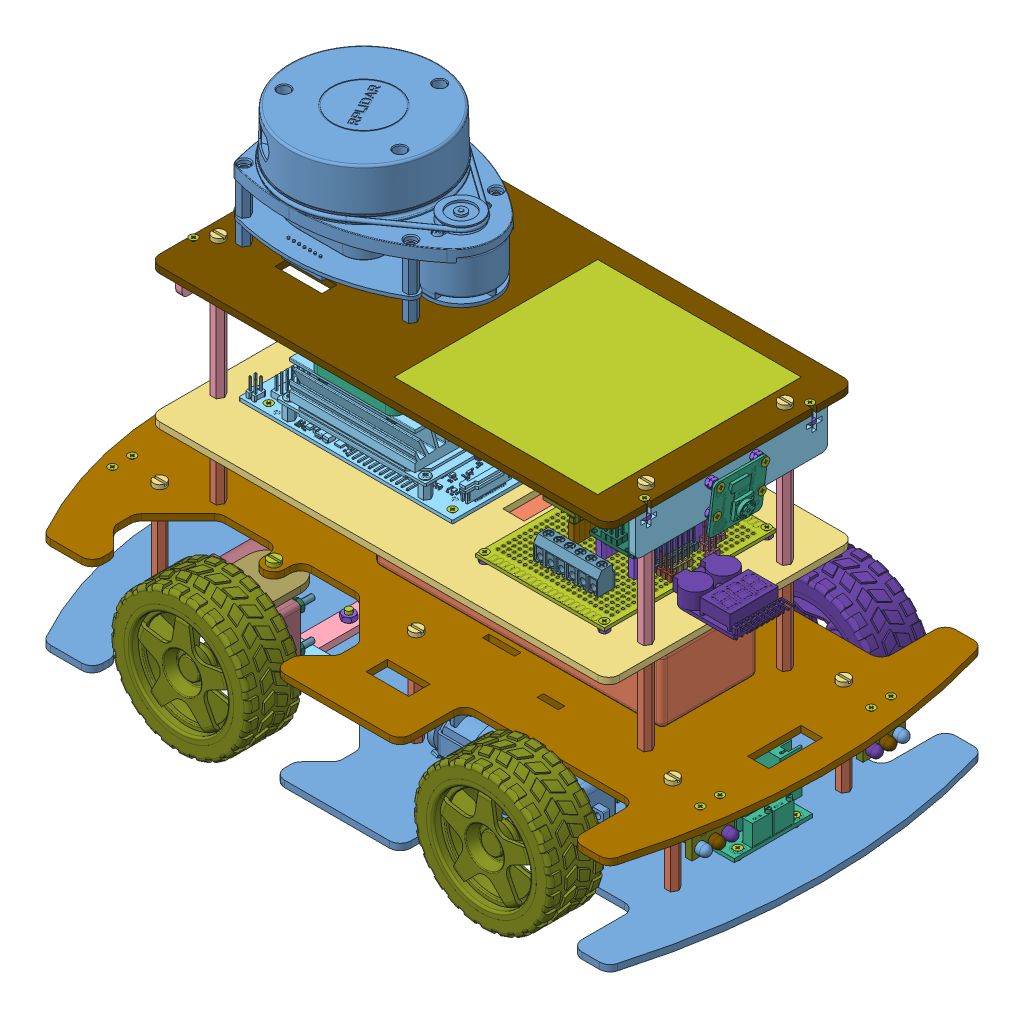
SolidWorks assembly Nigel - Motion Analysis, configuration Default. Lengths in mm. (continued)
Mates (geometry in assembly coordinates): (continued)
- Coincident280: coincident: circle of Platform 2-1; cone of M2x10 Bolt-16 through (137.5 46.8 -44.6) axis (0 -1 0)
- Concentric255: concentric: cylinder of M2x10 Bolt-16 through (137.5 47.6723 -44.6) axis (0 1 0) radius 1; cylinder of M2 Nut-16 through (137.5 40.5 -44.6) axis (0 -1 0) radius 1
- Coincident281: coincident: plane of LED Mount-4 through (139 40.5 -40) normal (0 -1 0); plane of M2 Nut-16 through (137.5 40.5 -44.6) normal (0 1 0)
- Concentric256: concentric: cylinder of Platform 3-1 through (-80 89 29) axis (0 -1 0) radius 1.1; cylinder of M2x10 Bolt-17 through (-80 94.4673 29) axis (0 1 0) radius 1
- Coincident282: coincident: circle of Jetson Nano B01-1; cone of M2x10 Bolt-17 through (-80 93.595 29) axis (0 -1 0)
- Concentric257: concentric: cylinder of Platform 3-1 through (-80 89 -29) axis (0 -1 0) radius 1.1; cylinder of M2x10 Bolt-18 through (-80 94.4673 -29) axis (0 1 0) radius 1
- Coincident283: coincident: circle of Jetson Nano B01-1; cone of M2x10 Bolt-18 through (-80 93.595 -29) axis (0 -1 0)
- Concentric258: concentric: cylinder of Platform 3-1 through (6 89 29) axis (0 -1 0) radius 1.1; cylinder of M2x10 Bolt-19 through (6 94.4673 29) axis (0 1 0) radius 1
- Coincident284: coincident: circle of Jetson Nano B01-1; cone of M2x10 Bolt-19 through (6 93.595 29) axis (0 -1 0)
- Concentric259: concentric: cylinder of Platform 3-1 through (6 89 -29) axis (0 -1 0) radius 1.1; cylinder of M2x10 Bolt-20 through (6 94.4673 -29) axis (0 1 0) radius 1
- Coincident285: coincident: circle of Jetson Nano B01-1; cone of M2x10 Bolt-20 through (6 93.595 -29) axis (0 -1 0)
- Concentric260: concentric: cylinder of M2x10 Bolt-17 through (-80 94.4673 29) axis (0 1 0) radius 1; cylinder of M2 Nut-17 through (-80 86 29) axis (0 -1 0) radius 1
- Coincident286: coincident: plane of Platform 3-1 through (0 86 0) normal (0 -1 0); plane of M2 Nut-17 through (-80 86 29) normal (0 1 0)
- Concentric261: concentric: cylinder of M2x10 Bolt-18 through (-80 94.4673 -29) axis (0 1 0) radius 1; cylinder of M2 Nut-18 through (-80 86 -29) axis (0 -1 0) radius 1
- Coincident287: coincident: plane of Platform 3-1 through (0 86 0) normal (0 -1 0); plane of M2 Nut-18 through (-80 86 -29) normal (0 1 0)
- Concentric262: concentric: cylinder of M2x10 Bolt-19 through (6 94.4673 29) axis (0 1 0) radius 1; cylinder of M2 Nut-19 through (6 86 29) axis (0 -1 0) radius 1
- Coincident288: coincident: plane of Platform 3-1 through (0 86 0) normal (0 -1 0); plane of M2 Nut-19 through (6 86 29) normal (0 1 0)
- Concentric263: concentric: cylinder of M2x10 Bolt-20 through (6 94.4673 -29) axis (0 1 0) radius 1; cylinder of M2 Nut-20 through (6 86 -29) axis (0 -1 0) radius 1
- Coincident289: coincident: plane of Platform 3-1 through (0 86 0) normal (0 -1 0); plane of M2 Nut-20 through (6 86 -29) normal (0 1 0)
- Concentric264: concentric: cylinder of Platform 4-1 through (-100 152 32.5) axis (0 -1 0) radius 1.6; cylinder of M3x8 Bolt-17 through (-100 144 32.5) axis (0 1 0) radius 1.5
- Coincident290: coincident: plane of Platform 4-1 through (0 152 0) normal (0 1 0); plane of M3x8 Bolt-17 through (-100 152 32.5) normal (0 -1 0)
- Concentric265: concentric: cylinder of Platform 4-1 through (-100 152 -32.5) axis (0 -1 0) radius 1.6; cylinder of M3x8 Bolt-18 through (-100 144 -32.5) axis (0 1 0) radius 1.5
- Coincident291: coincident: plane of Platform 4-1 through (0 152 0) normal (0 1 0); plane of M3x8 Bolt-18 through (-100 152 -32.5) normal (0 -1 0)
- Concentric266: concentric: cylinder of Platform 4-1 through (100 152 32.5) axis (0 -1 0) radius 1.6; cylinder of M3x8 Bolt-19 through (100 144 32.5) axis (0 1 0) radius 1.5
- Coincident292: coincident: plane of Platform 4-1 through (0 152 0) normal (0 1 0); plane of M3x8 Bolt-19 through (100 152 32.5) normal (0 -1 0)
- Concentric267: concentric: cylinder of Platform 4-1 through (100 152 -32.5) axis (0 -1 0) radius 1.6; cylinder of M3x8 Bolt-20 through (100 144 -32.5) axis (0 1 0) radius 1.5
- Coincident293: coincident: plane of Platform 4-1 through (0 152 0) normal (0 1 0); plane of M3x8 Bolt-20 through (100 152 -32.5) normal (0 -1 0)
- Concentric268: concentric: cylinder of Platform 4-1 through (-92.5 152 28) axis (0 -1 0) radius 1.35; cylinder of M2.5x8 Bolt-1 through (-92.5 147.1277 28) axis (0 -1 0) radius 1.25
- Coincident294: coincident: circle of Platform 4-1; cone of M2.5x8 Bolt-1 through (-92.5 148 28) axis (0 1 0)
- Concentric269: concentric: cylinder of Platform 4-1 through (-92.5 152 -28) axis (0 -1 0) radius 1.35; cylinder of M2.5x8 Bolt-2 through (-92.5 147.1277 -28) axis (0 -1 0) radius 1.25
- Coincident295: coincident: circle of Platform 4-1; cone of M2.5x8 Bolt-2 through (-92.5 148 -28) axis (0 1 0)
- Concentric270: concentric: cylinder of Platform 4-1 through (-22.5 152 20) axis (0 -1 0) radius 1.35; cylinder of M2.5x8 Bolt-3 through (-22.5 147.1277 20) axis (0 -1 0) radius 1.25
- Coincident296: coincident: circle of Platform 4-1; cone of M2.5x8 Bolt-3 through (-22.5 148 20) axis (0 1 0)
- Concentric271: concentric: cylinder of Platform 4-1 through (-22.5 152 -20) axis (0 -1 0) radius 1.35; cylinder of M2.5x8 Bolt-4 through (-22.5 147.1277 -20) axis (0 -1 0) radius 1.25
- Coincident297: coincident: circle of Platform 4-1; cone of M2.5x8 Bolt-4 through (-22.5 148 -20) axis (0 1 0)
- Concentric272: concentric: cylinder of RPLIDAR Adapter-1 through (-57.5 150.2284 -46.5) axis (0 -1 0) radius 1; cylinder of M2x10 Bolt-21 through (-57.5 144.1277 -46.5) axis (0 -1 0) radius 1
- Coincident298: coincident: circle of RPLIDAR Adapter-1; cone of M2x10 Bolt-21 through (-57.5 145 -46.5) axis (0 1 0)
- Concentric273: concentric: cylinder of RPLIDAR Adapter-1 through (-71.5 150.2284 -46.5) axis (0 -1 0) radius 1; cylinder of M2x10 Bolt-22 through (-71.5 144.1277 -46.5) axis (0 -1 0) radius 1
- Coincident299: coincident: circle of RPLIDAR Adapter-1; cone of M2x10 Bolt-22 through (-71.5 145 -46.5) axis (0 1 0)
- Concentric274: concentric: cylinder of RPLIDAR Adapter-1 through (-57.5 150.2284 -28) axis (0 -1 0) radius 1; cylinder of M2x10 Bolt-23 through (-57.5 144.1277 -28) axis (0 -1 0) radius 1
- Coincident300: coincident: circle of RPLIDAR Adapter-1; cone of M2x10 Bolt-23 through (-57.5 145 -28) axis (0 1 0)
- Concentric275: concentric: cylinder of RPLIDAR Adapter-1 through (-71.5 150.2284 -28) axis (0 -1 0) radius 1; cylinder of M2x10 Bolt-24 through (-71.5 144.1277 -28) axis (0 -1 0) radius 1
- Coincident301: coincident: circle of RPLIDAR Adapter-1; cone of M2x10 Bolt-24 through (-71.5 145 -28) axis (0 1 0)
- Concentric276: concentric: cylinder of M2x10 Bolt-21 through (-57.5 144.1277 -46.5) axis (0 -1 0) radius 1; cylinder of M2 Nut-21 through (-57.5 153.6 -46.5) axis (0 -1 0) radius 1
- Coincident302: coincident: plane of Platform 4-1 through (0 152 0) normal (0 1 0); plane of M2 Nut-21 through (-57.5 152 -46.5) normal (0 -1 0)
- Concentric277: concentric: cylinder of M2x10 Bolt-22 through (-71.5 144.1277 -46.5) axis (0 -1 0) radius 1; cylinder of M2 Nut-22 through (-71.5 153.6 -46.5) axis (0 -1 0) radius 1
- Coincident303: coincident: plane of Platform 4-1 through (0 152 0) normal (0 1 0); plane of M2 Nut-22 through (-71.5 152 -46.5) normal (0 -1 0)
- Concentric278: concentric: cylinder of M2x10 Bolt-23 through (-57.5 144.1277 -28) axis (0 -1 0) radius 1; cylinder of M2 Nut-23 through (-57.5 153.6 -28) axis (0 -1 0) radius 1
- Coincident304: coincident: plane of Platform 4-1 through (0 152 0) normal (0 1 0); plane of M2 Nut-23 through (-57.5 152 -28) normal (0 -1 0)
- Concentric279: concentric: cylinder of M2x10 Bolt-24 through (-71.5 144.1277 -28) axis (0 -1 0) radius 1; cylinder of M2 Nut-24 through (-71.5 153.6 -28) axis (0 -1 0) radius 1
- Coincident305: coincident: plane of Platform 4-1 through (0 152 0) normal (0 1 0); plane of M2 Nut-24 through (-71.5 152 -28) normal (0 -1 0)
- Tangent1: tangent: plane of Platform 4-1 through (-104.5 152 -39.8) normal (-1 0 0); cylinder of M2x10 Bolt-25 through (-105.5 153.6723 -38.7) axis (0 1 0) radius 1
- Distance33: distance = 0.1 mm: cylinder of M2x10 Bolt-25 through (-105.5 153.6723 -38.7) axis (0 1 0) radius 1; plane of Platform 4-1 through (-107.5 152 -39.8) normal (0 0 1)
- Distance34: distance = 3.7 mm: plane of M2x10 Bolt-25 through (-105.5 142.8 -38.7) normal (0 -1 0); plane of Front Camera Mount-1 through (-104.5 146.5 -37.6) normal (0 -1 0)
- Parallel23: parallel: plane of Front Camera Mount-1 through (-107.5 140.25 0) normal (-1 0 0); plane of M2x10 Bolt-25 through (-105.5 152.8 -38.7) normal (1 0 0)
- Tangent3: tangent: plane of Platform 4-1 through (-104.5 152 39.8) normal (-1 0 0); cylinder of M2x10 Bolt-26 through (-105.5 153.6723 38.7) axis (0 1 0) radius 1
- Distance35: distance = 0.1 mm: cylinder of M2x10 Bolt-26 through (-105.5 153.6723 38.7) axis (0 1 0) radius 1; plane of Platform 4-1 through (-104.5 152 37.6) normal (0 0 1)
- Distance36: distance = 3.7 mm: plane of M2x10 Bolt-26 through (-105.5 142.8 38.7) normal (0 -1 0); plane of Front Camera Mount-1 through (-104.5 146.5 42.3) normal (0 -1 0)
- Parallel24: parallel: plane of Front Camera Mount-1 through (-107.5 140.25 0) normal (-1 0 0); plane of M2x10 Bolt-26 through (-105.5 152.8 38.7) normal (1 0 0)
- Concentric280: concentric: cylinder of M2x10 Bolt-25 through (-105.5 153.6723 -38.7) axis (0 1 0) radius 1; cylinder of M2 Nut-25 through (-105.5 146.5 -38.7) axis (0 -1 0) radius 1
- Coincident310: coincident: plane of Front Camera Mount-1 through (-104.5 146.5 -37.6) normal (0 -1 0); plane of M2 Nut-25 through (-105.5 146.5 -38.7) normal (0 1 0)
- Concentric281: concentric: cylinder of M2x10 Bolt-26 through (-105.5 153.6723 38.7) axis (0 1 0) radius 1; cylinder of M2 Nut-26 through (-105.5 146.5 38.7) axis (0 -1 0) radius 1
- Coincident311: coincident: plane of Front Camera Mount-1 through (-104.5 146.5 42.3) normal (0 -1 0); plane of M2 Nut-26 through (-105.5 146.5 38.7) normal (0 1 0)
- Tangent5: tangent: plane of Platform 4-1 through (104.5 152 39.8) normal (1 0 0); cylinder of M2x10 Bolt-27 through (105.5 153.6723 38.7) axis (0 1 0) radius 1
- Distance37: distance = 0.1 mm: cylinder of M2x10 Bolt-27 through (105.5 153.6723 38.7) axis (0 1 0) radius 1; plane of Platform 4-1 through (107.5 152 39.8) normal (0 0 -1)
- Distance38: distance = 3.7 mm: plane of M2x10 Bolt-27 through (105.5 142.8 38.7) normal (0 -1 0); plane of Rear Camera Mount-1 through (107.5 146.5 37.6) normal (0 -1 0)
- Parallel25: parallel: plane of Rear Camera Mount-1 through (107.5 140.25 0) normal (1 0 0); plane of M2x10 Bolt-27 through (105.5 152.8 38.7) normal (1 0 0)
- Tangent7: tangent: plane of Platform 4-1 through (104.5 152 -39.8) normal (1 0 0); cylinder of M2x10 Bolt-28 through (105.5 153.6723 -38.7) axis (0 1 0) radius 1
- Distance39: distance = 0.1 mm: cylinder of M2x10 Bolt-28 through (105.5 153.6723 -38.7) axis (0 1 0) radius 1; plane of Platform 4-1 through (104.5 152 -37.6) normal (0 0 -1)
- Distance40: distance = 3.7 mm: plane of M2x10 Bolt-28 through (105.5 142.8 -38.7) normal (0 -1 0); plane of Rear Camera Mount-1 through (107.5 146.5 -42.3) normal (0 -1 0)
- Parallel26: parallel: plane of Rear Camera Mount-1 through (107.5 140.25 0) normal (1 0 0); plane of M2x10 Bolt-28 through (105.5 152.8 -38.7) normal (1 0 0)
- Concentric282: concentric: cylinder of M2x10 Bolt-27 through (105.5 153.6723 38.7) axis (0 1 0) radius 1; cylinder of M2 Nut-27 through (105.5 146.5 38.7) axis (0 -1 0) radius 1
- Coincident316: coincident: plane of Rear Camera Mount-1 through (107.5 146.5 37.6) normal (0 -1 0); plane of M2 Nut-27 through (105.5 146.5 38.7) normal (0 1 0)
- Concentric283: concentric: cylinder of M2x10 Bolt-28 through (105.5 153.6723 -38.7) axis (0 1 0) radius 1; cylinder of M2 Nut-28 through (105.5 146.5 -38.7) axis (0 -1 0) radius 1
- Coincident317: coincident: plane of Rear Camera Mount-1 through (107.5 146.5 -42.3) normal (0 -1 0); plane of M2 Nut-28 through (105.5 146.5 -38.7) normal (0 1 0)
- Concentric284: concentric: cylinder of Front Camera Mount-1 through (-104.5 146.5 -10.5) axis (-1 0 0) radius 1.1; cylinder of M2x10 Bolt-29 through (-113.8723 146.5 -10.5) axis (-1 0 0) radius 1
- Concentric285: concentric: cylinder of Front Camera Mount-1 through (-104.5 146.5 10.5) axis (-1 0 0) radius 1.1; cylinder of M2x10 Bolt-30 through (-113.8723 146.5 10.5) axis (-1 0 0) radius 1
- Concentric286: concentric: cylinder of Front Camera Mount-1 through (-104.5 134 -10.5) axis (-1 0 0) radius 1.1; cylinder of M2x10 Bolt-31 through (-112.2723 134 -10.5) axis (-1 0 0) radius 1
- Concentric287: concentric: cylinder of Front Camera Mount-1 through (-104.5 134 10.5) axis (-1 0 0) radius 1.1; cylinder of M2x10 Bolt-32 through (-112.2723 134 10.5) axis (-1 0 0) radius 1
- Concentric288: concentric: cylinder of M2x10 Bolt-29 through (-113.8723 146.5 -10.5) axis (-1 0 0) radius 1; cylinder of M2 Nut-29 through (-102.9 146.5 -10.5) axis (-1 0 0) radius 1
- Coincident322: coincident: plane of Front Camera Mount-1 through (-104.5 140.25 0) normal (1 0 0); plane of M2 Nut-29 through (-104.5 146.5 -10.5) normal (-1 0 0)
- Concentric289: concentric: cylinder of M2x10 Bolt-30 through (-113.8723 146.5 10.5) axis (-1 0 0) radius 1; cylinder of M2 Nut-30 through (-102.9 146.5 10.5) axis (-1 0 0) radius 1
- Coincident323: coincident: plane of Front Camera Mount-1 through (-104.5 140.25 0) normal (1 0 0); plane of M2 Nut-30 through (-104.5 146.5 10.5) normal (-1 0 0)
- Concentric290: concentric: cylinder of M2x10 Bolt-31 through (-112.2723 134 -10.5) axis (-1 0 0) radius 1; cylinder of M2 Nut-31 through (-102.9 134 -10.5) axis (-1 0 0) radius 1
- Coincident324: coincident: plane of Front Camera Mount-1 through (-104.5 140.25 0) normal (1 0 0); plane of M2 Nut-31 through (-104.5 134 -10.5) normal (-1 0 0)
- Concentric291: concentric: cylinder of M2x10 Bolt-32 through (-112.2723 134 10.5) axis (-1 0 0) radius 1; cylinder of M2 Nut-32 through (-102.9 134 10.5) axis (-1 0 0) radius 1
- Coincident325: coincident: plane of Front Camera Mount-1 through (-104.5 140.25 0) normal (1 0 0); plane of M2 Nut-32 through (-104.5 134 10.5) normal (-1 0 0)
- Concentric292: concentric: cylinder of Rear Camera Mount-1 through (107.5 146.5 10.5) axis (-1 0 0) radius 1.1; cylinder of M2x10 Bolt-33 through (113.8723 146.5 10.5) axis (1 0 0) radius 1
- Concentric293: concentric: cylinder of Rear Camera Mount-1 through (107.5 146.5 -10.5) axis (-1 0 0) radius 1.1; cylinder of M2x10 Bolt-34 through (113.8723 146.5 -10.5) axis (1 0 0) radius 1
- Concentric294: concentric: cylinder of Rear Camera Mount-1 through (107.5 134 10.5) axis (-1 0 0) radius 1.1; cylinder of M2x10 Bolt-35 through (112.2723 134 10.5) axis (1 0 0) radius 1
- Concentric295: concentric: cylinder of Rear Camera Mount-1 through (107.5 134 -10.5) axis (-1 0 0) radius 1.1; cylinder of M2x10 Bolt-36 through (112.2723 134 -10.5) axis (1 0 0) radius 1
- Concentric296: concentric: cylinder of M2x10 Bolt-33 through (113.8723 146.5 10.5) axis (1 0 0) radius 1; cylinder of M2 Nut-33 through (104.5 146.5 10.5) axis (-1 0 0) radius 1
- Coincident330: coincident: plane of Rear Camera Mount-1 through (104.5 140.25 0) normal (-1 0 0); plane of M2 Nut-33 through (104.5 146.5 10.5) normal (1 0 0)
- Concentric297: concentric: cylinder of M2x10 Bolt-34 through (113.8723 146.5 -10.5) axis (1 0 0) radius 1; cylinder of M2 Nut-34 through (104.5 146.5 -10.5) axis (-1 0 0) radius 1
- Coincident331: coincident: plane of Rear Camera Mount-1 through (104.5 140.25 0) normal (-1 0 0); plane of M2 Nut-34 through (104.5 146.5 -10.5) normal (1 0 0)
- Concentric298: concentric: cylinder of M2x10 Bolt-35 through (112.2723 134 10.5) axis (1 0 0) radius 1; cylinder of M2 Nut-35 through (104.5 134 10.5) axis (-1 0 0) radius 1
- Coincident332: coincident: plane of Rear Camera Mount-1 through (104.5 140.25 0) normal (-1 0 0); plane of M2 Nut-35 through (104.5 134 10.5) normal (1 0 0)
- Concentric299: concentric: cylinder of M2x10 Bolt-36 through (112.2723 134 -10.5) axis (1 0 0) radius 1; cylinder of M2 Nut-36 through (104.5 134 -10.5) axis (-1 0 0) radius 1
- Coincident333: coincident: plane of Rear Camera Mount-1 through (104.5 140.25 0) normal (-1 0 0); plane of M2 Nut-36 through (104.5 134 -10.5) normal (1 0 0)
- Concentric300: concentric: cylinder of Platform 3-1 through (-100 89 32.5) axis (0 -1 0) radius 1.6; cylinder of M3x60 M-F Standoff-1 through (-100 83 32.5) axis (0 1 0) radius 1.5
- Coincident334: coincident: plane of Platform 3-1 through (0 89 0) normal (0 1 0); plane of M3x60 M-F Standoff-1 through (-100 89 32.5) normal (0 -1 0)
- Concentric301: concentric: cylinder of Platform 4-1 through (-100 152 32.5) axis (0 -1 0) radius 1.6; cylinder of M3x60 M-F Standoff-1 through (-100 129 32.5) axis (0 1 0) radius 1.5
- Coincident335: coincident: plane of Platform 4-1 through (0 149 0) normal (0 -1 0); plane of M3x60 M-F Standoff-1 through (18.5533 149 -128.4176) normal (0 1 0)
- Concentric302: concentric: cylinder of Platform 3-1 through (-100 89 -32.5) axis (0 -1 0) radius 1.6; cylinder of M3x60 M-F Standoff-2 through (-100 83 -32.5) axis (0 1 0) radius 1.5
- Coincident337: coincident: plane of Platform 3-1 through (0 89 0) normal (0 1 0); plane of M3x60 M-F Standoff-2 through (-100 89 -32.5) normal (0 -1 0)
- Concentric303: concentric: cylinder of Platform 4-1 through (-100 152 -32.5) axis (0 -1 0) radius 1.6; cylinder of M3x60 M-F Standoff-2 through (-100 129 -32.5) axis (0 1 0) radius 1.5
- Concentric304: concentric: cylinder of Platform 3-1 through (100 89 32.5) axis (0 -1 0) radius 1.6; cylinder of M3x60 M-F Standoff-3 through (100 83 32.5) axis (0 1 0) radius 1.5
- Coincident338: coincident: plane of Platform 3-1 through (0 89 0) normal (0 1 0); plane of M3x60 M-F Standoff-3 through (100 89 32.5) normal (0 -1 0)
- Concentric305: concentric: cylinder of Platform 3-1 through (100 89 -32.5) axis (0 -1 0) radius 1.6; cylinder of M3x60 M-F Standoff-4 through (100 83 -32.5) axis (0 1 0) radius 1.5
- Coincident339: coincident: plane of Platform 3-1 through (0 89 0) normal (0 1 0); plane of M3x60 M-F Standoff-4 through (100 89 -32.5) normal (0 -1 0)
- Concentric306: concentric: cylinder of Platform 1-1 through (-15 3 21) axis (0 -1 0) radius 1.6; cylinder of M4x5 Spacer-1 through (-15 8 21) axis (0 -1 0) radius 2
- Coincident340: coincident: plane of Platform 1-1 through (-150 3 0) normal (0 1 0); plane of M4x5 Spacer-1 through (-15 3 21) normal (0 -1 0)
- Coincident341: coincident: plane of Motor Driver-1 through (-3 8 0) normal (0 -1 0); plane of M4x5 Spacer-1 through (-15 8 21) normal (0 1 0)
- Concentric307: concentric: cylinder of Platform 1-1 through (-15 3 -21) axis (0 -1 0) radius 1.6; cylinder of M4x5 Spacer-2 through (-15 8 -21) axis (0 -1 0) radius 2
- Coincident342: coincident: plane of Platform 1-1 through (-150 3 0) normal (0 1 0); plane of M4x5 Spacer-2 through (-15 3 -21) normal (0 -1 0)
- Concentric308: concentric: cylinder of Platform 1-1 through (9 3 21) axis (0 -1 0) radius 1.6; cylinder of M4x5 Spacer-3 through (9 8 21) axis (0 -1 0) radius 2
- Coincident343: coincident: plane of Platform 1-1 through (-150 3 0) normal (0 1 0); plane of M4x5 Spacer-3 through (9 3 21) normal (0 -1 0)
- Concentric309: concentric: cylinder of Motor Driver-1 through (9 9.5 -21) axis (0 -1 0) radius 1.6; cylinder of M4x5 Spacer-4 through (9 8 -21) axis (0 -1 0) radius 2
- Coincident344: coincident: plane of Platform 1-1 through (-150 3 0) normal (0 1 0); plane of M4x5 Spacer-4 through (9 3 -21) normal (0 -1 0)
- Concentric310: concentric: cylinder of Platform 1-1 through (-15 3 21) axis (0 -1 0) radius 1.6; cylinder of M3x14 Bolt-3 through (-15 -4.5 21) axis (0 1 0) radius 1.5
- Coincident345: coincident: plane of Motor Driver-1 through (-3 9.5 0) normal (0 1 0); plane of M3x14 Bolt-3 through (-15 9.5 21) normal (0 -1 0)
- Concentric311: concentric: cylinder of Platform 1-1 through (-15 3 -21) axis (0 -1 0) radius 1.6; cylinder of M3x14 Bolt-4 through (-15 -4.5 -21) axis (0 1 0) radius 1.5
- Coincident346: coincident: plane of Motor Driver-1 through (-3 9.5 0) normal (0 1 0); plane of M3x14 Bolt-4 through (-15 9.5 -21) normal (0 -1 0)
- Concentric312: concentric: cylinder of M3x14 Bolt-5 through (9 -4.5 21) axis (0 1 0) radius 1.5; cylinder of Platform 1-1 through (9 3 21) axis (0 -1 0) radius 1.6
- Coincident347: coincident: plane of Motor Driver-1 through (-3 9.5 0) normal (0 1 0); plane of M3x14 Bolt-5 through (9 9.5 21) normal (0 -1 0)
- Concentric313: concentric: cylinder of Platform 1-1 through (9 3 -21) axis (0 -1 0) radius 1.6; cylinder of M3x14 Bolt-6 through (9 -4.5 -21) axis (0 1 0) radius 1.5
- Coincident348: coincident: plane of Motor Driver-1 through (-3 9.5 0) normal (0 1 0); plane of M3x14 Bolt-6 through (9 9.5 -21) normal (0 -1 0)
- Concentric314: concentric: cylinder of M3x14 Bolt-3 through (-15 -4.5 21) axis (0 1 0) radius 1.5; cylinder of M3 Nut-15 through (-15 0 21) axis (0 -1 0) radius 1.5
- Coincident349: coincident: plane of Platform 1-1 through (-150 0 0) normal (0 -1 0); plane of M3 Nut-15 through (-15 0 21) normal (0 1 0)
- Concentric315: concentric: cylinder of M3x14 Bolt-4 through (-15 -4.5 -21) axis (0 1 0) radius 1.5; cylinder of M3 Nut-16 through (-15 0 -21) axis (0 -1 0) radius 1.5
- Coincident350: coincident: plane of Platform 1-1 through (-150 0 0) normal (0 -1 0); plane of M3 Nut-16 through (-15 0 -21) normal (0 1 0)
- Concentric316: concentric: cylinder of M3x14 Bolt-5 through (9 -4.5 21) axis (0 1 0) radius 1.5; cylinder of M3 Nut-17 through (9 0 21) axis (0 -1 0) radius 1.5
- Coincident351: coincident: plane of Platform 1-1 through (-150 0 0) normal (0 -1 0); plane of M3 Nut-17 through (9 0 21) normal (0 1 0)
- Concentric317: concentric: cylinder of M3x14 Bolt-6 through (9 -4.5 -21) axis (0 1 0) radius 1.5; cylinder of M3 Nut-18 through (9 0 -21) axis (0 -1 0) radius 1.5
- Coincident352: coincident: plane of Platform 1-1 through (-150 0 0) normal (0 -1 0); plane of M3 Nut-18 through (9 0 -21) normal (0 1 0)
- Concentric318: concentric: cylinder of Platform 3-1 through (30 89 38) axis (0 -1 0) radius 1.1; cylinder of Auxillary Board-1/PCB-1 through (30 92.1 38) axis (0 -1 0) radius 1.15
- Concentric319: concentric: cylinder of Platform 3-1 through (30 89 -38) axis (0 -1 0) radius 1.1; cylinder of Auxillary Board-1/PCB-1 through (30 92.1 -38) axis (0 -1 0) radius 1.15
- Concentric320: concentric: cylinder of Jetson Nano B01-1 through (-54 119.7762 28.3) axis (0 1 0) radius 1.35; cylinder of 4020 DC Fan-1 through (-54 119.2762 28.3) axis (0 -1 0) radius 1.5
- Concentric321: concentric: cylinder of Jetson Nano B01-1 through (-22 119.7762 28.3) axis (0 1 0) radius 1.35; cylinder of 4020 DC Fan-1 through (-22 119.2762 28.3) axis (0 -1 0) radius 1.5
- Coincident353: coincident: plane of Jetson Nano B01-1 through (-5.2 119.7762 24.216) normal (0 1 0); plane of 4020 DC Fan-1 through (-38 119.7762 12.3) normal (0 -1 0)
- Concentric322: concentric: cylinder of 4020 DC Fan-1 through (-54 119.2762 28.3) axis (0 -1 0) radius 1.5; cylinder of M2.5x25 Bolt-5 through (-54 114.7762 28.3) axis (0 1 0) radius 1.25
- Coincident354: coincident: plane of 4020 DC Fan-1 through (-54 139.7762 -3.7) normal (0 1 0); plane of M2.5x25 Bolt-5 through (-54 139.7762 28.3) normal (0 -1 0)
- Concentric323: concentric: cylinder of 4020 DC Fan-1 through (-22 119.2762 28.3) axis (0 -1 0) radius 1.5; cylinder of M2.5x25 Bolt-6 through (-22 114.7762 28.3) axis (0 1 0) radius 1.25
- Coincident355: coincident: plane of 4020 DC Fan-1 through (-54 139.7762 -3.7) normal (0 1 0); plane of M2.5x25 Bolt-6 through (-22 139.7762 28.3) normal (0 -1 0)
- Concentric324: concentric: cylinder of 4020 DC Fan-1 through (-54 119.2762 -3.7) axis (0 -1 0) radius 1.5; cylinder of M2.5x25 Bolt-7 through (-54 114.7762 -3.7) axis (0 1 0) radius 1.25
- Coincident356: coincident: plane of 4020 DC Fan-1 through (-54 139.7762 -3.7) normal (0 1 0); plane of M2.5x25 Bolt-7 through (-54 139.7762 -3.7) normal (0 -1 0)
- Concentric325: concentric: cylinder of 4020 DC Fan-1 through (-22 119.2762 -3.7) axis (0 -1 0) radius 1.5; cylinder of M2.5x25 Bolt-8 through (-22 114.7762 -3.7) axis (0 1 0) radius 1.25
- Coincident357: coincident: plane of 4020 DC Fan-1 through (-54 139.7762 -3.7) normal (0 1 0); plane of M2.5x25 Bolt-8 through (-22 139.7762 -3.7) normal (0 -1 0)
- Concentric326: concentric: cylinder of M2.5 Nut-5 through (-54 118.2762 28.3) axis (0 -1 0) radius 1.25; cylinder of M2.5x25 Bolt-5 through (-54 114.7762 28.3) axis (0 1 0) radius 1.25
- Concentric327: concentric: cylinder of M2.5x25 Bolt-6 through (-22 114.7762 28.3) axis (0 1 0) radius 1.25; cylinder of M2.5 Nut-6 through (-22 118.2762 28.3) axis (0 -1 0) radius 1.25
- Concentric328: concentric: cylinder of M2.5x25 Bolt-7 through (-54 114.7762 -3.7) axis (0 1 0) radius 1.25; cylinder of M2.5 Nut-7 through (-54 118.2762 -3.7) axis (0 -1 0) radius 1.25
- Concentric329: concentric: cylinder of M2.5x25 Bolt-8 through (-22 114.7762 -3.7) axis (0 1 0) radius 1.25; cylinder of M2.5 Nut-8 through (-22 118.2762 -3.7) axis (0 -1 0) radius 1.25
- Coincident358: coincident: plane of Jetson Nano B01-1 through (-5.2 118.2762 32.8141) normal (0 -1 0); plane of M2.5 Nut-5 through (-54 118.2762 28.3) normal (0 1 0)
- Coincident359: coincident: plane of Jetson Nano B01-1 through (-5.2 118.2762 32.8141) normal (0 -1 0); plane of M2.5 Nut-6 through (-22 118.2762 28.3) normal (0 1 0)
- Coincident360: coincident: plane of Jetson Nano B01-1 through (-5.2 118.2762 0.7859) normal (0 -1 0); plane of M2.5 Nut-7 through (-54 118.2762 -3.7) normal (0 1 0)
- Coincident361: coincident: plane of Jetson Nano B01-1 through (-5.2 118.2762 0.7859) normal (0 -1 0); plane of M2.5 Nut-8 through (-22 118.2762 -3.7) normal (0 1 0)
- Concentric330: concentric: cylinder of Platform 3-1 through (30 89 38) axis (0 -1 0) radius 1.1; cylinder of M2x10 Bolt-37 through (30 93.7223 38) axis (0 1 0) radius 1
- Coincident362: coincident: circle of Auxillary Board-1/PCB-1; cone of M2x10 Bolt-37 through (30 92.85 38) axis (0 -1 0)
- Concentric331: concentric: cylinder of Platform 3-1 through (30 89 -38) axis (0 -1 0) radius 1.1; cylinder of M2x10 Bolt-38 through (30 93.7223 -38) axis (0 1 0) radius 1
- Coincident363: coincident: circle of Auxillary Board-1/PCB-1; cone of M2x10 Bolt-38 through (30 92.85 -38) axis (0 -1 0)
- Concentric332: concentric: cylinder of Platform 3-1 through (86 89 38) axis (0 -1 0) radius 1.1; cylinder of M2x10 Bolt-39 through (86 93.7223 38) axis (0 1 0) radius 1
- Coincident364: coincident: circle of Auxillary Board-1/PCB-1; cone of M2x10 Bolt-39 through (86 92.85 38) axis (0 -1 0)
- Concentric333: concentric: cylinder of Platform 3-1 through (86 89 -38) axis (0 -1 0) radius 1.1; cylinder of M2x10 Bolt-40 through (86 93.7223 -38) axis (0 1 0) radius 1
- Coincident365: coincident: circle of Auxillary Board-1/PCB-1; cone of M2x10 Bolt-40 through (86 92.85 -38) axis (0 -1 0)
- Concentric334: concentric: cylinder of M2x10 Bolt-37 through (30 93.7223 38) axis (0 1 0) radius 1; cylinder of M2 Nut-37 through (30 86 38) axis (0 -1 0) radius 1
- Coincident366: coincident: plane of Platform 3-1 through (0 86 0) normal (0 -1 0); plane of M2 Nut-37 through (30 86 38) normal (0 1 0)
- Concentric335: concentric: cylinder of M2x10 Bolt-38 through (30 93.7223 -38) axis (0 1 0) radius 1; cylinder of M2 Nut-38 through (30 86 -38) axis (0 -1 0) radius 1
- Coincident367: coincident: plane of Platform 3-1 through (0 86 0) normal (0 -1 0); plane of M2 Nut-38 through (30 86 -38) normal (0 1 0)
- Concentric336: concentric: cylinder of M2x10 Bolt-39 through (86 93.7223 38) axis (0 1 0) radius 1; cylinder of M2 Nut-39 through (86 86 38) axis (0 -1 0) radius 1
- Coincident368: coincident: plane of Platform 3-1 through (0 86 0) normal (0 -1 0); plane of M2 Nut-39 through (86 86 38) normal (0 1 0)
- Concentric337: concentric: cylinder of M2x10 Bolt-40 through (86 93.7223 -38) axis (0 1 0) radius 1; cylinder of M2 Nut-40 through (86 86 -38) axis (0 -1 0) radius 1
- Coincident369: coincident: plane of Platform 3-1 through (0 86 0) normal (0 -1 0); plane of M2 Nut-40 through (86 86 -38) normal (0 1 0)
- Concentric338: concentric: cylinder of Platform 2-1 through (-100 46 32.5) axis (0 -1 0) radius 1.6; cylinder of M3x40 F-F Standoff-7 through (-100 41.7574 32.5) axis (0 1 0) radius 1.5
- Coincident370: coincident: plane of Platform 2-1 through (-150 46 0) normal (0 1 0); plane of M3x40 F-F Standoff-7 through (-100 46 32.5) normal (0 -1 0)
- Concentric339: concentric: cylinder of Platform 3-1 through (-100 89 32.5) axis (0 -1 0) radius 1.6; cylinder of M3x40 F-F Standoff-7 through (-100 41.7574 32.5) axis (0 1 0) radius 1.5
- Coincident371: coincident: plane of Platform 3-1 through (0 86 0) normal (0 -1 0); plane of M3x40 F-F Standoff-7 through (18.5533 86 -128.4176) normal (0 1 0)
- Concentric340: concentric: cylinder of Platform 2-1 through (-100 46 -32.5) axis (0 -1 0) radius 1.6; cylinder of M3x40 F-F Standoff-8 through (-100 41.7574 -32.5) axis (0 1 0) radius 1.5
- Coincident372: coincident: plane of Platform 2-1 through (-150 46 0) normal (0 1 0); plane of M3x40 F-F Standoff-8 through (-100 46 -32.5) normal (0 -1 0)
- Concentric341: concentric: cylinder of Platform 3-1 through (-100 89 -32.5) axis (0 -1 0) radius 1.6; cylinder of M3x40 F-F Standoff-8 through (-100 41.7574 -32.5) axis (0 1 0) radius 1.5
- Coincident373: coincident: plane of Platform 2-1 through (-150 46 0) normal (0 1 0); plane of M3x40 F-F Standoff-9 through (100 46 32.5) normal (0 -1 0)
- Concentric342: concentric: cylinder of Platform 2-1 through (100 46 32.5) axis (0 -1 0) radius 1.6; cylinder of M3x40 F-F Standoff-9 through (100 41.7574 32.5) axis (0 1 0) radius 1.5
- Coincident374: coincident: plane of Platform 2-1 through (-150 46 0) normal (0 1 0); plane of M3x40 F-F Standoff-10 through (100 46 -32.5) normal (0 -1 0)
- Concentric343: concentric: cylinder of Platform 2-1 through (100 46 -32.5) axis (0 -1 0) radius 1.6; cylinder of M3x40 F-F Standoff-10 through (100 41.7574 -32.5) axis (0 1 0) radius 1.5
- Coincident379: coincident: plane of Platform 3-1 through (0 89 0) normal (0 1 0); plane of LiPo Battery Voltage Tester-1 through (101.9765 89 1.3) normal (0 -1 0)
- Distance43: distance = 1 mm: plane of LiPo Battery Voltage Tester-1 through (89.1 94.03 0) normal (-1 0 0); plane of Auxillary Board-1/PCB-1 through (88.1 92.1 40.1) normal (1 0 0)
- Distance44: distance = 45.5 mm: plane of LiPo Battery Voltage Tester-1 through (120.6 91 12) normal (0 0 1); plane of Platform 3-1 through (-107.5 89 57.5) normal (0 0 1)
- Concentric348: concentric: cylinder of M2x10 Bolt-21 through (-57.5 144.1277 -46.5) axis (0 -1 0) radius 1; cylinder of M2 Nut-45 through (-57.5 149 -46.5) axis (0 -1 0) radius 1
- Coincident381: coincident: plane of Platform 4-1 through (0 149 0) normal (0 -1 0); plane of M2 Nut-45 through (-57.5 149 -46.5) normal (0 1 0)
- Concentric349: concentric: cylinder of M2x10 Bolt-22 through (-71.5 144.1277 -46.5) axis (0 -1 0) radius 1; cylinder of M2 Nut-46 through (-71.5 149 -46.5) axis (0 -1 0) radius 1
- Coincident382: coincident: plane of Platform 4-1 through (0 149 0) normal (0 -1 0); plane of M2 Nut-46 through (-71.5 149 -46.5) normal (0 1 0)
- Coincident380: coincident: plane of Auxillary Board-1/PCB-1 through (58 90.6 0) normal (0 -1 0); plane of M2 Nut-47 through (30 90.6 38) normal (0 1 0)
- Concentric354: concentric: cylinder of M2x10 Bolt-37 through (30 93.7223 38) axis (0 1 0) radius 1; cylinder of M2 Nut-47 through (30 90.6 38) axis (0 -1 0) radius 1
- Coincident387: coincident: plane of Platform 3-1 through (0 89 0) normal (0 1 0); plane of M2 Nut-47 through (30 89 38) normal (0 -1 0)
- Concentric355: concentric: cylinder of M2x10 Bolt-38 through (30 93.7223 -38) axis (0 1 0) radius 1; cylinder of M2 Nut-48 through (30 90.6 -38) axis (0 -1 0) radius 1
- Coincident388: coincident: plane of Platform 3-1 through (0 89 0) normal (0 1 0); plane of M2 Nut-48 through (30 89 -38) normal (0 -1 0)
- Concentric356: concentric: cylinder of M2x10 Bolt-39 through (86 93.7223 38) axis (0 1 0) radius 1; cylinder of M2 Nut-49 through (86 90.6 38) axis (0 -1 0) radius 1
- Coincident389: coincident: plane of Platform 3-1 through (0 89 0) normal (0 1 0); plane of M2 Nut-49 through (86 89 38) normal (0 -1 0)
- Concentric357: concentric: cylinder of M2x10 Bolt-40 through (86 93.7223 -38) axis (0 1 0) radius 1; cylinder of M2 Nut-50 through (86 90.6 -38) axis (0 -1 0) radius 1
- Coincident390: coincident: plane of Platform 3-1 through (0 89 0) normal (0 1 0); plane of M2 Nut-50 through (86 89 -38) normal (0 -1 0)
- Concentric358: concentric: cylinder of M2x10 Bolt-23 through (-57.5 144.1277 -28) axis (0 -1 0) radius 1; cylinder of M2 Nut-51 through (-57.5 149 -28) axis (0 -1 0) radius 1
- Coincident391: coincident: plane of Platform 4-1 through (0 149 0) normal (0 -1 0); plane of M2 Nut-51 through (-57.5 149 -28) normal (0 1 0)
- Concentric359: concentric: cylinder of M2x10 Bolt-24 through (-71.5 144.1277 -28) axis (0 -1 0) radius 1; cylinder of M2 Nut-52 through (-71.5 149 -28) axis (0 -1 0) radius 1
- Coincident392: coincident: plane of Platform 4-1 through (0 149 0) normal (0 -1 0); plane of M2 Nut-52 through (-71.5 149 -28) normal (0 1 0)
- Concentric360: concentric: cylinder of Front Camera Mount-1 through (-104.5 146.5 -10.5) axis (-1 0 0) radius 1.1; cylinder of M2 Nut-53 through (-109.1 146.5 -10.5) axis (1 0 0) radius 1
- Coincident393: coincident: plane of Front Camera Mount-1 through (-107.5 140.25 0) normal (-1 0 0); plane of M2 Nut-53 through (-107.5 146.5 -10.5) normal (1 0 0)
- Concentric361: concentric: cylinder of Front Camera Mount-1 through (-104.5 146.5 10.5) axis (-1 0 0) radius 1.1; cylinder of M2 Nut-54 through (-109.1 146.5 10.5) axis (1 0 0) radius 1
- Coincident394: coincident: plane of Front Camera Mount-1 through (-107.5 140.25 0) normal (-1 0 0); plane of M2 Nut-54 through (-107.5 146.5 10.5) normal (1 0 0)
- Concentric362: concentric: cylinder of Front Camera Mount-1 through (-104.5 134 -10.5) axis (-1 0 0) radius 1.1; cylinder of M2 Nut-55 through (-109.1 134 -10.5) axis (1 0 0) radius 1
- Coincident395: coincident: plane of Front Camera Mount-1 through (-107.5 140.25 0) normal (-1 0 0); plane of M2 Nut-55 through (-107.5 134 -10.5) normal (1 0 0)
- Concentric363: concentric: cylinder of Front Camera Mount-1 through (-104.5 134 10.5) axis (-1 0 0) radius 1.1; cylinder of M2 Nut-56 through (-109.1 134 10.5) axis (1 0 0) radius 1
- Coincident396: coincident: plane of Front Camera Mount-1 through (-107.5 140.25 0) normal (-1 0 0); plane of M2 Nut-56 through (-107.5 134 10.5) normal (1 0 0)
- Concentric364: concentric: cylinder of M2 Nut-53 through (-109.1 146.5 -10.5) axis (1 0 0) radius 1; cylinder of M2 Nut-57 through (-110.7 146.5 -10.5) axis (1 0 0) radius 1
- Coincident397: coincident: plane of M2 Nut-53 through (-109.1 146.5 -10.5) normal (-1 0 0); plane of M2 Nut-57 through (-109.1 146.5 -10.5) normal (1 0 0)
- Concentric365: concentric: cylinder of M2 Nut-54 through (-109.1 146.5 10.5) axis (1 0 0) radius 1; cylinder of M2 Nut-58 through (-110.7 146.5 10.5) axis (1 0 0) radius 1
- Coincident398: coincident: plane of M2 Nut-54 through (-109.1 146.5 10.5) normal (-1 0 0); plane of M2 Nut-58 through (-109.1 146.5 10.5) normal (1 0 0)
- Coincident406: coincident: plane of Raspberry Pi Camera V2.1-1 through (-109.6979 136.6712 0) normal (0.991907 0.126964 0); point of M2 Nut-56
- Coincident407: coincident: plane of Raspberry Pi Camera V2.1-1 through (-109.6979 136.6712 0) normal (0.991907 0.126964 0); point of M2 Nut-58
- Coincident408: coincident: plane of Raspberry Pi Camera V2.1-1 through (-109.6979 136.6712 0) normal (0.991907 0.126964 0); point of M2 Nut-55
- Coincident410: coincident: plane of Raspberry Pi Camera V2.1-1 through (-109.6979 136.6712 0) normal (0.991907 0.126964 0); point of M2 Nut-57
- Distance53: distance = 0.05 mm: line of Front Camera Mount-1 through (-107.5 149 -37.6) axis (0 0 1); plane of Raspberry Pi Camera V2.1-1 through (-111.2215 148.5741 10.5) normal (-0.126964 0.991907 0)
- Distance49: distance = 32.5 mm: plane of Raspberry Pi Camera V2.1-1 through (-110.9676 146.5902 -12.5) normal (0 0 -1); plane of Front Camera Mount-1 through (-104.5 131.5 -45) normal (0 0 -1)
- Distance47: distance = 1.5 mm: plane of M2x10 Bolt-29 through (-103 146.5 -10.5) normal (1 0 0); plane of Front Camera Mount-1 through (-104.5 140.25 0) normal (1 0 0)
- Distance50: distance = 1.5 mm: plane of M2x10 Bolt-30 through (-103 146.5 10.5) normal (1 0 0); plane of Front Camera Mount-1 through (-104.5 140.25 0) normal (1 0 0)
- Distance51: distance = 3.1 mm: plane of M2x10 Bolt-31 through (-101.4 134 -10.5) normal (1 0 0); plane of Front Camera Mount-1 through (-104.5 140.25 0) normal (1 0 0)
- Distance52: distance = 3.1 mm: plane of M2x10 Bolt-32 through (-101.4 134 10.5) normal (1 0 0); plane of Front Camera Mount-1 through (-104.5 140.25 0) normal (1 0 0)
- Concentric367: concentric: cylinder of Rear Camera Mount-1 through (107.5 146.5 10.5) axis (-1 0 0) radius 1.1; cylinder of M2 Nut-59 through (107.5 146.5 10.5) axis (1 0 0) radius 1
- Coincident422: coincident: plane of Rear Camera Mount-1 through (107.5 140.25 0) normal (1 0 0); plane of M2 Nut-59 through (107.5 146.5 10.5) normal (-1 0 0)
- Concentric368: concentric: cylinder of Rear Camera Mount-1 through (107.5 146.5 -10.5) axis (-1 0 0) radius 1.1; cylinder of M2 Nut-60 through (107.5 146.5 -10.5) axis (1 0 0) radius 1
- Coincident423: coincident: plane of Rear Camera Mount-1 through (107.5 140.25 0) normal (1 0 0); plane of M2 Nut-60 through (107.5 146.5 -10.5) normal (-1 0 0)
- Concentric369: concentric: cylinder of Rear Camera Mount-1 through (107.5 134 10.5) axis (-1 0 0) radius 1.1; cylinder of M2 Nut-61 through (107.5 134 10.5) axis (1 0 0) radius 1
- Coincident424: coincident: plane of Rear Camera Mount-1 through (107.5 140.25 0) normal (1 0 0); plane of M2 Nut-61 through (107.5 134 10.5) normal (-1 0 0)
- Concentric370: concentric: cylinder of Rear Camera Mount-1 through (107.5 134 -10.5) axis (-1 0 0) radius 1.1; cylinder of M2 Nut-62 through (107.5 134 -10.5) axis (1 0 0) radius 1
- Coincident425: coincident: plane of Rear Camera Mount-1 through (107.5 140.25 0) normal (1 0 0); plane of M2 Nut-62 through (107.5 134 -10.5) normal (-1 0 0)
- Concentric371: concentric: cylinder of M2 Nut-59 through (107.5 146.5 10.5) axis (1 0 0) radius 1; cylinder of M2 Nut-63 through (109.1 146.5 10.5) axis (1 0 0) radius 1
- Coincident426: coincident: plane of M2 Nut-59 through (109.1 146.5 10.5) normal (1 0 0); plane of M2 Nut-63 through (109.1 146.5 10.5) normal (-1 0 0)
- Concentric372: concentric: cylinder of M2 Nut-60 through (107.5 146.5 -10.5) axis (1 0 0) radius 1; cylinder of M2 Nut-64 through (109.1 146.5 -10.5) axis (1 0 0) radius 1
- Coincident427: coincident: plane of M2 Nut-60 through (109.1 146.5 -10.5) normal (1 0 0); plane of M2 Nut-64 through (109.1 146.5 -10.5) normal (-1 0 0)
- Coincident428: coincident: plane of Raspberry Pi Camera V2.1-2 through (109.6979 136.6712 0) normal (-0.991907 0.126964 0); point of M2 Nut-62
- Coincident429: coincident: plane of Raspberry Pi Camera V2.1-2 through (109.6979 136.6712 0) normal (-0.991907 0.126964 0); point of M2 Nut-64
- Coincident430: coincident: plane of Raspberry Pi Camera V2.1-2 through (109.6979 136.6712 0) normal (-0.991907 0.126964 0); point of M2 Nut-61
- Coincident431: coincident: plane of Raspberry Pi Camera V2.1-2 through (109.6979 136.6712 0) normal (-0.991907 0.126964 0); point of M2 Nut-63
- Distance54: distance = 0.05 mm: line of Rear Camera Mount-1 through (107.5 149 -37.6) axis (0 0 1); plane of Raspberry Pi Camera V2.1-2 through (111.2215 148.5741 -10.5) normal (0.126964 0.991907 0)
- Distance55: distance = 32.5 mm: plane of Raspberry Pi Camera V2.1-2 through (110.9676 146.5902 12.5) normal (0 0 1); plane of Rear Camera Mount-1 through (107.5 131.5 45) normal (0 0 1)
- Distance56: distance = 1.5 mm: plane of M2x10 Bolt-33 through (103 146.5 10.5) normal (-1 0 0); plane of Rear Camera Mount-1 through (104.5 140.25 0) normal (-1 0 0)
- Distance57: distance = 1.5 mm: plane of M2x10 Bolt-34 through (103 146.5 -10.5) normal (-1 0 0); plane of Rear Camera Mount-1 through (104.5 140.25 0) normal (-1 0 0)
- Distance58: distance = 3.1 mm: plane of M2x10 Bolt-35 through (101.4 134 10.5) normal (-1 0 0); plane of Rear Camera Mount-1 through (104.5 140.25 0) normal (-1 0 0)
- Distance59: distance = 3.1 mm: plane of M2x10 Bolt-36 through (101.4 134 -10.5) normal (-1 0 0); plane of Rear Camera Mount-1 through (104.5 140.25 0) normal (-1 0 0)
